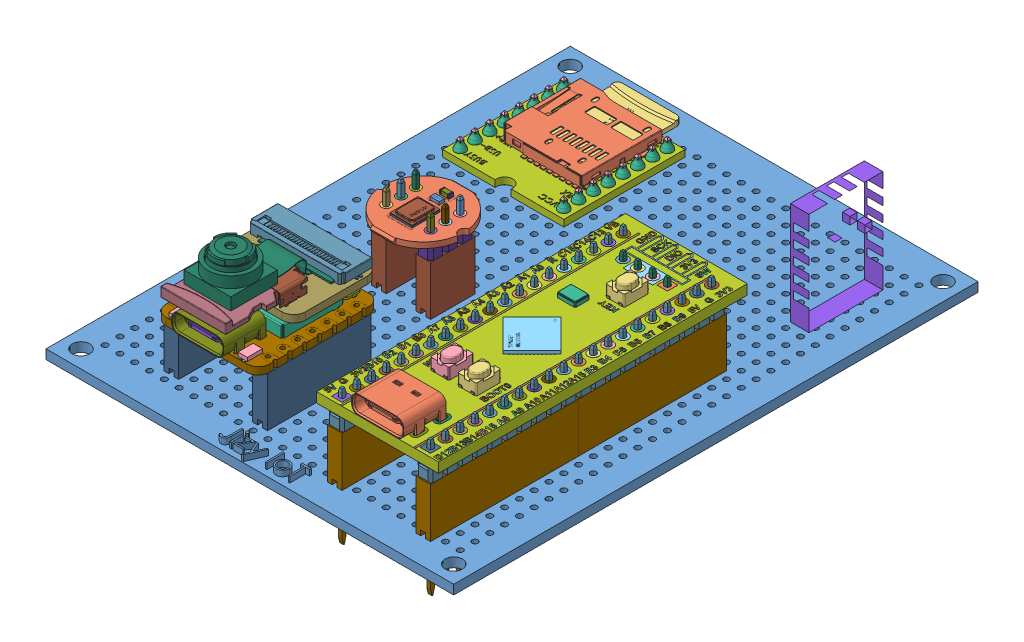
SolidWorks assembly 3D_Final, configuration Default. Lengths in mm.
Overall size (70 34.34 90).
331 component instances, 245 part files, 43 mates.
Components (placement in the parent):
- BoardDong7x9-1: BoardDong7x9 [Default] at (35 1.6 45) x (0 0 -1) z (0 1 0) size (90 70 2.6)
- blackpill v2.0 swi.STEP-1: blackpill v2.0 swi.STEP [Default] at (52.8 12.64 59.37) x (0 0 -1) z (0 1 0) size (53 20.9 10.45)
  - blackpill v2.0.step.STEP-1: blackpill v2.0.step.STEP [Default] at origin size (53 20.9 4.92)
    - USB Type C Port (SMD Type).step.STEP-1: USB Type C Port (SMD Type).step.STEP [Default] at (-19.2 0 3.305) x (0 -1 0) z (0 0 -1) size (8.94 7.9 4.2)
    - PTS810 SJK 250 SMTR LFS--3DModel-STEP-1.step.STEP-1: PTS810 SJK 250 SMTR LFS--3DModel-STEP-1.step.STEP [Default] at (14.5 -1.8498 1.7) x (1 0 0) z (0 -1 0) size (4.6 2.51 3.2)
    - PTS810 SJK 250 SMTR LFS--3DModel-STEP-1.step.STEP-2: PTS810 SJK 250 SMTR LFS--3DModel-STEP-1.step.STEP [Default] at (-11.4 -2.3498 1.7) x (1 0 0) z (0 -1 0) size (4.6 2.51 3.2)
    - PTS810 SJK 250 SMTR LFS--3DModel-STEP-1 v2(Mirror).step.STEP-1: PTS810 SJK 250 SMTR LFS--3DModel-STEP-1 v2(Mirror).step.STEP [Default] at (-11.4 2.3498 1.7) x (1 0 0) z (0 -1 0) size (4.6 2.51 3.2)
    - STM32F411CEU6.step.STEP-1: STM32F411CEU6.step.STEP [Default] at (0 0 1.7) x (-0.707107 -0.707107 0) z (-0.707107 0.707107 0) size (7 0.6 7)
    - ECS-135.60-12-33Q-JES-TR.step.STEP-1: ECS-135.60-12-33Q-JES-TR.step.STEP [Default] at (9.3867 2.3215 1.7) x (0 -1 0) z (-1 0 0) size (3.2 0.8 2.5)
    - DIY_black_pill.step.STEP-1: DIY_black_pill.step.STEP [Default] at origin size (53 20.9 1.7)
    - DIY_black_pill-0.step.STEP-1: DIY_black_pill-0.step.STEP [Default] at origin size (1.8 1.8 1.72)
    - DIY_black_pill-1.step.STEP-1: DIY_black_pill-1.step.STEP [Default] at origin size (1.8 1.8 1.72)
    - DIY_black_pill-2.step.STEP-1: DIY_black_pill-2.step.STEP [Default] at origin size (1.8 1.8 1.72)
    - DIY_black_pill-3.step.STEP-1: DIY_black_pill-3.step.STEP [Default] at origin size (1.8 1.8 1.72)
    - DIY_black_pill-4.step.STEP-1: DIY_black_pill-4.step.STEP [Default] at origin size (1.8 1.8 1.72)
    - DIY_black_pill-5.step.STEP-1: DIY_black_pill-5.step.STEP [Default] at origin size (1.8 1.8 1.72)
    - DIY_black_pill-6.step.STEP-1: DIY_black_pill-6.step.STEP [Default] at origin size (1.8 1.8 1.72)
    - DIY_black_pill-7.step.STEP-1: DIY_black_pill-7.step.STEP [Default] at origin size (1.8 1.8 1.72)
    - DIY_black_pill-8.step.STEP-1: DIY_black_pill-8.step.STEP [Default] at origin size (1.8 1.8 1.72)
    - DIY_black_pill-9.step.STEP-1: DIY_black_pill-9.step.STEP [Default] at origin size (1.8 1.8 1.72)
    - DIY_black_pill-10.step.STEP-1: DIY_black_pill-10.step.STEP [Default] at origin size (1.8 1.8 1.72)
    - DIY_black_pill-11.step.STEP-1: DIY_black_pill-11.step.STEP [Default] at origin size (1.8 1.8 1.72)
    - DIY_black_pill-12.step.STEP-1: DIY_black_pill-12.step.STEP [Default] at origin size (1.8 1.8 1.72)
    - DIY_black_pill-13.step.STEP-1: DIY_black_pill-13.step.STEP [Default] at origin size (1.8 1.8 1.72)
    - DIY_black_pill-14.step.STEP-1: DIY_black_pill-14.step.STEP [Default] at origin size (1.8 1.8 1.72)
    - DIY_black_pill-15.step.STEP-1: DIY_black_pill-15.step.STEP [Default] at origin size (1.8 1.8 1.72)
    - DIY_black_pill-16.step.STEP-1: DIY_black_pill-16.step.STEP [Default] at origin size (1.8 1.8 1.72)
    - DIY_black_pill-17.step.STEP-1: DIY_black_pill-17.step.STEP [Default] at origin size (1.8 1.8 1.72)
    - DIY_black_pill-18.step.STEP-1: DIY_black_pill-18.step.STEP [Default] at origin size (1.8 1.8 1.72)
    - DIY_black_pill-19.step.STEP-1: DIY_black_pill-19.step.STEP [Default] at origin size (1.8 1.8 1.72)
    - DIY_black_pill-20.step.STEP-1: DIY_black_pill-20.step.STEP [Default] at origin size (1.8 1.8 1.72)
    - DIY_black_pill-21.step.STEP-1: DIY_black_pill-21.step.STEP [Default] at origin size (1.8 1.8 1.72)
    - DIY_black_pill-22.step.STEP-1: DIY_black_pill-22.step.STEP [Default] at origin size (1.8 1.8 1.72)
    - DIY_black_pill-23.step.STEP-1: DIY_black_pill-23.step.STEP [Default] at origin size (1.8 1.8 1.72)
    - DIY_black_pill-24.step.STEP-1: DIY_black_pill-24.step.STEP [Default] at origin size (1.8 1.8 1.72)
    - DIY_black_pill-25.step.STEP-1: DIY_black_pill-25.step.STEP [Default] at origin size (1.8 1.8 1.72)
    - DIY_black_pill-26.step.STEP-1: DIY_black_pill-26.step.STEP [Default] at origin size (1.8 1.8 1.72)
    - DIY_black_pill-27.step.STEP-1: DIY_black_pill-27.step.STEP [Default] at origin size (1.8 1.8 1.72)
    - DIY_black_pill-28.step.STEP-1: DIY_black_pill-28.step.STEP [Default] at origin size (1.8 1.8 1.72)
    - DIY_black_pill-29.step.STEP-1: DIY_black_pill-29.step.STEP [Default] at origin size (1.8 1.8 1.72)
    - DIY_black_pill-30.step.STEP-1: DIY_black_pill-30.step.STEP [Default] at origin size (1.8 1.8 1.72)
    - DIY_black_pill-31.step.STEP-1: DIY_black_pill-31.step.STEP [Default] at origin size (1.8 1.8 1.72)
    - DIY_black_pill-32.step.STEP-1: DIY_black_pill-32.step.STEP [Default] at origin size (1.8 1.8 1.72)
    - DIY_black_pill-33.step.STEP-1: DIY_black_pill-33.step.STEP [Default] at origin size (1.8 1.8 1.72)
    - DIY_black_pill-34.step.STEP-1: DIY_black_pill-34.step.STEP [Default] at origin size (1.8 1.8 1.72)
    - DIY_black_pill-35.step.STEP-1: DIY_black_pill-35.step.STEP [Default] at origin size (1.8 1.8 1.72)
    - DIY_black_pill-36.step.STEP-1: DIY_black_pill-36.step.STEP [Default] at origin size (1.8 1.8 1.72)
    - DIY_black_pill-37.step.STEP-1: DIY_black_pill-37.step.STEP [Default] at origin size (1.8 1.8 1.72)
    - DIY_black_pill-38.step.STEP-1: DIY_black_pill-38.step.STEP [Default] at origin size (1.8 1.8 1.72)
    - DIY_black_pill-39.step.STEP-1: DIY_black_pill-39.step.STEP [Default] at origin size (1.8 1.8 1.72)
    - DIY_black_pill-40.step.STEP-1: DIY_black_pill-40.step.STEP [Default] at origin size (51.2 0.3 0.01)
    - DIY_black_pill-41.step.STEP-1: DIY_black_pill-41.step.STEP [Default] at origin size (51.2 0.3 0.01)
    - DIY_black_pill-42.step.STEP-1: DIY_black_pill-42.step.STEP [Default] at origin size (0.93 1 0.01)
    - DIY_black_pill-43.step.STEP-1: DIY_black_pill-43.step.STEP [Default] at origin size (0.94 1.03 0.01)
    - DIY_black_pill-44.step.STEP-1: DIY_black_pill-44.step.STEP [Default] at origin size (0.93 1 0.01)
    - DIY_black_pill-45.step.STEP-1: DIY_black_pill-45.step.STEP [Default] at origin size (0.67 1.02 0.01)
    - DIY_black_pill-46.step.STEP-1: DIY_black_pill-46.step.STEP [Default] at origin size (0.66 1.02 0.01)
    - DIY_black_pill-47.step.STEP-1: DIY_black_pill-47.step.STEP [Default] at origin size (0.84 1 0.01)
    - DIY_black_pill-48.step.STEP-1: DIY_black_pill-48.step.STEP [Default] at origin size (0.67 1.02 0.01)
    - DIY_black_pill-49.step.STEP-1: DIY_black_pill-49.step.STEP [Default] at origin size (0.84 1.01 0.01)
    - DIY_black_pill-50.step.STEP-1: DIY_black_pill-50.step.STEP [Default] at origin size (0.72 1.01 0.01)
    - DIY_black_pill-51.step.STEP-1: DIY_black_pill-51.step.STEP [Default] at origin size (0.84 1 0.01)
    - DIY_black_pill-52.step.STEP-1: DIY_black_pill-52.step.STEP [Default] at origin size (0.67 1 0.01)
    - DIY_black_pill-53.step.STEP-1: DIY_black_pill-53.step.STEP [Default] at origin size (1 1 0.01)
    - DIY_black_pill-54.step.STEP-1: DIY_black_pill-54.step.STEP [Default] at origin size (0.44 1 0.01)
    - DIY_black_pill-55.step.STEP-1: DIY_black_pill-55.step.STEP [Default] at origin size (0.44 1 0.01)
    - DIY_black_pill-56.step.STEP-1: DIY_black_pill-56.step.STEP [Default] at origin size (1 1 0.01)
    - DIY_black_pill-57.step.STEP-1: DIY_black_pill-57.step.STEP [Default] at origin size (0.44 1 0.01)
    - DIY_black_pill-58.step.STEP-1: DIY_black_pill-58.step.STEP [Default] at origin size (0.67 1.02 0.01)
    - DIY_black_pill-59.step.STEP-1: DIY_black_pill-59.step.STEP [Default] at origin size (0.66 1.02 0.01)
    - DIY_black_pill-60.step.STEP-1: DIY_black_pill-60.step.STEP [Default] at origin size (0.67 1 0.01)
    - DIY_black_pill-61.step.STEP-1: DIY_black_pill-61.step.STEP [Default] at origin size (0.84 1 0.01)
    - DIY_black_pill-62.step.STEP-1: DIY_black_pill-62.step.STEP [Default] at origin size (0.44 1 0.01)
    - DIY_black_pill-63.step.STEP-1: DIY_black_pill-63.step.STEP [Default] at origin size (0.66 1.02 0.01)
    - DIY_black_pill-64.step.STEP-1: DIY_black_pill-64.step.STEP [Default] at origin size (0.44 1 0.01)
    - DIY_black_pill-65.step.STEP-1: DIY_black_pill-65.step.STEP [Default] at origin size (0.84 1 0.01)
    - DIY_black_pill-66.step.STEP-1: DIY_black_pill-66.step.STEP [Default] at origin size (0.72 1 0.01)
    - DIY_black_pill-67.step.STEP-1: DIY_black_pill-67.step.STEP [Default] at origin size (0.44 1 0.01)
    - DIY_black_pill-68.step.STEP-1: DIY_black_pill-68.step.STEP [Default] at origin size (0.84 1 0.01)
    - DIY_black_pill-69.step.STEP-1: DIY_black_pill-69.step.STEP [Default] at origin size (1 1 0.01)
    - DIY_black_pill-70.step.STEP-1: DIY_black_pill-70.step.STEP [Default] at origin size (1 1 0.01)
    - DIY_black_pill-71.step.STEP-1: DIY_black_pill-71.step.STEP [Default] at origin size (0.65 1.02 0.01)
    - DIY_black_pill-72.step.STEP-1: DIY_black_pill-72.step.STEP [Default] at origin size (0.44 1 0.01)
    - DIY_black_pill-73.step.STEP-1: DIY_black_pill-73.step.STEP [Default] at origin size (1 1 0.01)
    - DIY_black_pill-74.step.STEP-1: DIY_black_pill-74.step.STEP [Default] at origin size (0.67 1 0.01)
    - DIY_black_pill-75.step.STEP-1: DIY_black_pill-75.step.STEP [Default] at origin size (0.44 1 0.01)
    - DIY_black_pill-76.step.STEP-1: DIY_black_pill-76.step.STEP [Default] at origin size (1 1 0.01)
    - DIY_black_pill-77.step.STEP-1: DIY_black_pill-77.step.STEP [Default] at origin size (0.66 1.02 0.01)
    - DIY_black_pill-78.step.STEP-1: DIY_black_pill-78.step.STEP [Default] at origin size (0.84 1.01 0.01)
    - DIY_black_pill-79.step.STEP-1: DIY_black_pill-79.step.STEP [Default] at origin size (0.67 1.01 0.01)
    - DIY_black_pill-80.step.STEP-1: DIY_black_pill-80.step.STEP [Default] at origin size (0.84 1 0.01)
    - DIY_black_pill-81.step.STEP-1: DIY_black_pill-81.step.STEP [Default] at origin size (0.66 0.99 0.01)
    - DIY_black_pill-82.step.STEP-1: DIY_black_pill-82.step.STEP [Default] at origin size (0.84 1 0.01)
    - DIY_black_pill-83.step.STEP-1: DIY_black_pill-83.step.STEP [Default] at origin size (0.84 1 0.01)
    - DIY_black_pill-84.step.STEP-1: DIY_black_pill-84.step.STEP [Default] at origin size (0.67 1 0.01)
    - DIY_black_pill-85.step.STEP-1: DIY_black_pill-85.step.STEP [Default] at origin size (0.66 1.02 0.01)
    - DIY_black_pill-86.step.STEP-1: DIY_black_pill-86.step.STEP [Default] at origin size (0.66 1.02 0.01)
    - DIY_black_pill-87.step.STEP-1: DIY_black_pill-87.step.STEP [Default] at origin size (0.67 1 0.01)
    - DIY_black_pill-88.step.STEP-1: DIY_black_pill-88.step.STEP [Default] at origin size (0.44 1 0.01)
    - DIY_black_pill-89.step.STEP-1: DIY_black_pill-89.step.STEP [Default] at origin size (0.84 1 0.01)
    - DIY_black_pill-90.step.STEP-1: DIY_black_pill-90.step.STEP [Default] at origin size (1 1 0.01)
    - DIY_black_pill-91.step.STEP-1: DIY_black_pill-91.step.STEP [Default] at origin size (0.84 1 0.01)
    - DIY_black_pill-92.step.STEP-1: DIY_black_pill-92.step.STEP [Default] at origin size (0.44 1 0.01)
    - DIY_black_pill-93.step.STEP-1: DIY_black_pill-93.step.STEP [Default] at origin size (0.87 1.03 0.01)
    - DIY_black_pill-94.step.STEP-1: DIY_black_pill-94.step.STEP [Default] at origin size (0.44 1 0.01)
    - DIY_black_pill-95.step.STEP-1: DIY_black_pill-95.step.STEP [Default] at origin size (0.44 1 0.01)
    - DIY_black_pill-96.step.STEP-1: DIY_black_pill-96.step.STEP [Default] at origin size (0.9 1 0.01)
    - DIY_black_pill-97.step.STEP-1: DIY_black_pill-97.step.STEP [Default] at origin size (0.65 1.02 0.01)
    - DIY_black_pill-98.step.STEP-1: DIY_black_pill-98.step.STEP [Default] at origin size (1 1 0.01)
    - DIY_black_pill-99.step.STEP-1: DIY_black_pill-99.step.STEP [Default] at origin size (0.72 1 0.01)
    - DIY_black_pill-100.step.STEP-1: DIY_black_pill-100.step.STEP [Default] at origin size (1 1 0.01)
    - DIY_black_pill-101.step.STEP-1: DIY_black_pill-101.step.STEP [Default] at origin size (0.67 1.02 0.01)
    - DIY_black_pill-102.step.STEP-1: DIY_black_pill-102.step.STEP [Default] at origin size (0.65 1.02 0.01)
    - DIY_black_pill-103.step.STEP-1: DIY_black_pill-103.step.STEP [Default] at origin size (1 1 0.01)
    - DIY_black_pill-104.step.STEP-1: DIY_black_pill-104.step.STEP [Default] at origin size (0.84 1 0.01)
    - DIY_black_pill-105.step.STEP-1: DIY_black_pill-105.step.STEP [Default] at origin size (0.84 1 0.01)
    - DIY_black_pill-106.step.STEP-1: DIY_black_pill-106.step.STEP [Default] at origin size (0.65 1.02 0.01)
    - DIY_black_pill-107.step.STEP-1: DIY_black_pill-107.step.STEP [Default] at origin size (0.66 1.02 0.01)
    - DIY_black_pill-108.step.STEP-1: DIY_black_pill-108.step.STEP [Default] at origin size (0.66 1.02 0.01)
    - DIY_black_pill-109.step.STEP-1: DIY_black_pill-109.step.STEP [Default] at origin size (0.67 1 0.01)
    - DIY_black_pill-110.step.STEP-1: DIY_black_pill-110.step.STEP [Default] at origin size (0.93 1 0.01)
    - DIY_black_pill-111.step.STEP-1: DIY_black_pill-111.step.STEP [Default] at origin size (0.94 1.03 0.01)
    - DIY_black_pill-112.step.STEP-1: DIY_black_pill-112.step.STEP [Default] at origin size (0.93 1 0.01)
    - DIY_black_pill-113.step.STEP-1: DIY_black_pill-113.step.STEP [Default] at origin size (0.44 1 0.01)
    - DIY_black_pill-114.step.STEP-1: DIY_black_pill-114.step.STEP [Default] at origin size (0.84 1 0.01)
    - DIY_black_pill-115.step.STEP-1: DIY_black_pill-115.step.STEP [Default] at origin size (0.67 1 0.01)
    - DIY_black_pill-116.step.STEP-1: DIY_black_pill-116.step.STEP [Default] at origin size (0.44 1 0.01)
    - DIY_black_pill-117.step.STEP-1: DIY_black_pill-117.step.STEP [Default] at origin size (0.66 0.99 0.01)
    - DIY_black_pill-118.step.STEP-1: DIY_black_pill-118.step.STEP [Default] at origin size (0.84 1 0.01)
    - DIY_black_pill-119.step.STEP-1: DIY_black_pill-119.step.STEP [Default] at origin size (1 1 0.01)
    - DIY_black_pill-120.step.STEP-1: DIY_black_pill-120.step.STEP [Default] at origin size (0.67 1 0.01)
    - DIY_black_pill-121.step.STEP-1: DIY_black_pill-121.step.STEP [Default] at origin size (1 1 0.01)
    - DIY_black_pill-122.step.STEP-1: DIY_black_pill-122.step.STEP [Default] at origin size (0.66 1.02 0.01)
    - DIY_black_pill-123.step.STEP-1: DIY_black_pill-123.step.STEP [Default] at origin size (1 1 0.01)
    - DIY_black_pill-124.step.STEP-1: DIY_black_pill-124.step.STEP [Default] at origin size (0.67 1 0.01)
    - DIY_black_pill-125.step.STEP-1: DIY_black_pill-125.step.STEP [Default] at origin size (0.87 1.03 0.01)
    - DIY_black_pill-126.step.STEP-1: DIY_black_pill-126.step.STEP [Default] at origin size (0.72 1 0.01)
    - DIY_black_pill-127.step.STEP-1: DIY_black_pill-127.step.STEP [Default] at origin size (0.66 1.02 0.01)
    - DIY_black_pill-128.step.STEP-1: DIY_black_pill-128.step.STEP [Default] at origin size (0.87 1.03 0.01)
    - DIY_black_pill-129.step.STEP-1: DIY_black_pill-129.step.STEP [Default] at origin size (0.93 1 0.01)
    - DIY_black_pill-130.step.STEP-1: DIY_black_pill-130.step.STEP [Default] at origin size (0.44 1 0.01)
    - DIY_black_pill-131.step.STEP-1: DIY_black_pill-131.step.STEP [Default] at origin size (2.55 1.5 1.72)
    - DIY_black_pill-132.step.STEP-1: DIY_black_pill-132.step.STEP [Default] at origin size (2.6 1.5 1.72)
    - DIY_black_pill-133.step.STEP-1: DIY_black_pill-133.step.STEP [Default] at origin size (2.55 1.5 1.72)
    - DIY_black_pill-134.step.STEP-1: DIY_black_pill-134.step.STEP [Default] at origin size (2.6 1.5 1.72)
    - DIY_black_pill-135.step.STEP-1: DIY_black_pill-135.step.STEP [Default] at origin size (1 1 0.01)
    - DIY_black_pill-136.step.STEP-1: DIY_black_pill-136.step.STEP [Default] at origin size (0.67 1.01 0.01)
    - DIY_black_pill-137.step.STEP-1: DIY_black_pill-137.step.STEP [Default] at origin size (1.8 1.8 1.72)
    - DIY_black_pill-138.step.STEP-1: DIY_black_pill-138.step.STEP [Default] at origin size (1.8 1.8 1.72)
    - DIY_black_pill-139.step.STEP-1: DIY_black_pill-139.step.STEP [Default] at origin size (1.8 1.8 1.72)
    - DIY_black_pill-140.step.STEP-1: DIY_black_pill-140.step.STEP [Default] at origin size (1.8 1.8 1.72)
    - DIY_black_pill-141.step.STEP-1: DIY_black_pill-141.step.STEP [Default] at origin size (8.17 10.16 0.01)
    - DIY_black_pill-142.step.STEP-1: DIY_black_pill-142.step.STEP [Default] at origin size (1.31 1 0.01)
    - DIY_black_pill-143.step.STEP-1: DIY_black_pill-143.step.STEP [Default] at origin size (0.93 1 0.01)
    - DIY_black_pill-144.step.STEP-1: DIY_black_pill-144.step.STEP [Default] at origin size (0.84 1 0.01)
    - DIY_black_pill-145.step.STEP-1: DIY_black_pill-145.step.STEP [Default] at origin size (0.2 1 0.01)
    - DIY_black_pill-146.step.STEP-1: DIY_black_pill-146.step.STEP [Default] at origin size (0.87 1.03 0.01)
    - DIY_black_pill-147.step.STEP-1: DIY_black_pill-147.step.STEP [Default] at origin size (0.94 1.03 0.01)
    - DIY_black_pill-148.step.STEP-1: DIY_black_pill-148.step.STEP [Default] at origin size (0.79 1 0.01)
    - DIY_black_pill-149.step.STEP-1: DIY_black_pill-149.step.STEP [Default] at origin size (0.84 1 0.01)
    - DIY_black_pill-150.step.STEP-1: DIY_black_pill-150.step.STEP [Default] at origin size (0.9 1 0.01)
    - DIY_black_pill-151.step.STEP-1: DIY_black_pill-151.step.STEP [Default] at origin size (0.81 1.03 0.01)
    - DIY_black_pill-152.step.STEP-1: DIY_black_pill-152.step.STEP [Default] at origin size (0.97 1.03 0.01)
    - DIY_black_pill-153.step.STEP-1: DIY_black_pill-153.step.STEP [Default] at origin size (0.66 1.02 0.01)
    - DIY_black_pill-154.step.STEP-1: DIY_black_pill-154.step.STEP [Default] at origin size (0.66 1.02 0.01)
    - DIY_black_pill-155.step.STEP-1: DIY_black_pill-155.step.STEP [Default] at origin size (0.81 1.03 0.01)
    - DIY_black_pill-156.step.STEP-1: DIY_black_pill-156.step.STEP [Default] at origin size (0.9 1 0.01)
    - DIY_black_pill-157.step.STEP-1: DIY_black_pill-157.step.STEP [Default] at origin size (0.81 1.03 0.01)
    - DIY_black_pill-158.step.STEP-1: DIY_black_pill-158.step.STEP [Default] at origin size (0.97 1.03 0.01)
    - DIY_black_pill-159.step.STEP-1: DIY_black_pill-159.step.STEP [Default] at origin size (0.97 1.03 0.01)
    - DIY_black_pill-160.step.STEP-1: DIY_black_pill-160.step.STEP [Default] at origin size (1.01 0.91 0.01)
    - DIY_black_pill-161.step.STEP-1: DIY_black_pill-161.step.STEP [Default] at origin size (1 0.94 0.01)
    - DIY_black_pill-162.step.STEP-1: DIY_black_pill-162.step.STEP [Default] at origin size (1 0.77 0.01)
    - DIY_black_pill-163.step.STEP-1: DIY_black_pill-163.step.STEP [Default] at origin size (0.79 1 0.01)
    - DIY_black_pill-164.step.STEP-1: DIY_black_pill-164.step.STEP [Default] at origin size (0.65 1.02 0.01)
    - DIY_black_pill-165.step.STEP-1: DIY_black_pill-165.step.STEP [Default] at origin size (0.84 1 0.01)
    - DIY_black_pill-166.step.STEP-1: DIY_black_pill-166.step.STEP [Default] at origin size (0.79 1 0.01)
    - DIY_black_pill-167.step.STEP-1: DIY_black_pill-167.step.STEP [Default] at origin size (0.79 1 0.01)
  - 1x20 Male Pin Header.STEP-1: 1x20 Male Pin Header.STEP [Default] at (23.26 -7.6 0) x (-1 0 0) z (0 -1 0) size (50.8 8.54 2.5)
  - 1x20 Male Pin Header.STEP-2: 1x20 Male Pin Header.STEP [Default] at (23.26 7.6 0) x (-1 0 0) z (0 -1 0) size (50.8 8.54 2.5)
  - 1x4 Male Pin Header.STEP-1: 1x4 Male Pin Header.STEP [Default] at (19.45 -3.81 0) x (0 1 0) z (-1 0 0) size (10.17 8.54 2.5)
- Seeed Studio XIAO-ESP32-S3-Sense-1: Seeed Studio XIAO-ESP32-S3-Sense [Default] at (16.1886 10.35 72.4693) x (0 0 1) z (-1 0 0) size (24.36 13.98 17.79)
  - Seeed Studio XIAO-ESP32-S3-Sense.step-1: Seeed Studio XIAO-ESP32-S3-Sense.step [Default] at origin size (24.36 13.98 17.79)
    - Seeed Studio XIAO-ESP32-S3 (Sense).step-1: Seeed Studio XIAO-ESP32-S3 (Sense).step [Default] at origin size (22.49 4.48 17.79)
      - USB TYPE C PORT.step-1: USB TYPE C PORT.step [Default] at (4.3161 13.395 -12.1571) x (0 0 -1) z (0 -1 0) size (8.94 7.9 4.2)
        - USB TYPE C PORT (1).step-1: USB TYPE C PORT (1).step [Default] at (-3.0192 1.0963 5.395) size (8.94 7.9 4.2)
          - BOSS-EXTRUDE14_8_.step-1: BOSS-EXTRUDE14_8_.step [Default] at (-3.0192 1.0963 5.395) size (0.6 1 0.3)
          - BOSS-EXTRUDE7_4_.step-1: BOSS-EXTRUDE7_4_.step [Default] at (-3.0192 1.0963 5.395) size (0.3 3.78 0.75)
          - BOSS-EXTRUDE7_3_.step-1: BOSS-EXTRUDE7_3_.step [Default] at (-3.0192 1.0963 5.395) size (0.3 3.78 0.75)
          - BOSS-EXTRUDE14_4_.step-1: BOSS-EXTRUDE14_4_.step [Default] at (-3.0192 1.0963 5.395) size (0.3 1 0.3)
          - BOSS-EXTRUDE14_2_.step-1: BOSS-EXTRUDE14_2_.step [Default] at (-3.0192 1.0963 5.395) size (0.6 1 0.3)
          - BOSS-EXTRUDE14_11_.step-1: BOSS-EXTRUDE14_11_.step [Default] at (-3.0192 1.0963 5.395) size (0.3 1 0.3)
          - BOSS-EXTRUDE7_7_.step-1: BOSS-EXTRUDE7_7_.step [Default] at (-3.0192 1.0963 5.395) size (0.3 3.78 0.75)
          - BOSS-EXTRUDE14_9_.step-1: BOSS-EXTRUDE14_9_.step [Default] at (-3.0192 1.0963 5.395) size (0.3 1 0.3)
          - BOSS-EXTRUDE14_3_.step-1: BOSS-EXTRUDE14_3_.step [Default] at (-3.0192 1.0963 5.395) size (0.3 1 0.3)
          - BOSS-EXTRUDE14_7_.step-1: BOSS-EXTRUDE14_7_.step [Default] at (-3.0192 1.0963 5.395) size (0.6 1 0.3)
          - MIRROR2.step-1: MIRROR2.step [Default] at (-3.0192 1.0963 5.395) size (6.7 4.6 0.7)
          - BOSS-EXTRUDE14_5_.step-1: BOSS-EXTRUDE14_5_.step [Default] at (-3.0192 1.0963 5.395) size (0.3 1 0.3)
          - BOSS-EXTRUDE14_12_.step-1: BOSS-EXTRUDE14_12_.step [Default] at (-3.0192 1.0963 5.395) size (0.3 1 0.3)
          - BOSS-EXTRUDE7_8_.step-1: BOSS-EXTRUDE7_8_.step [Default] at (-3.0192 1.0963 5.395) size (0.3 3.78 0.75)
          - BOSS-EXTRUDE7_1_.step-1: BOSS-EXTRUDE7_1_.step [Default] at (-3.0192 1.0963 5.395) size (0.3 3.78 0.75)
          - BOSS-EXTRUDE14_10_.step-1: BOSS-EXTRUDE14_10_.step [Default] at (-3.0192 1.0963 5.395) size (0.3 1 0.3)
          - BOSS-EXTRUDE7_9_.step-1: BOSS-EXTRUDE7_9_.step [Default] at (-3.0192 1.0963 5.395) size (0.3 3.78 0.75)
          - BOSS-EXTRUDE14_6_.step-1: BOSS-EXTRUDE14_6_.step [Default] at (-3.0192 1.0963 5.395) size (0.6 1 0.3)
          - CHAMFER9.step-1: CHAMFER9.step [Default] at (-3.0192 1.0963 5.395) size (8.94 7.3 4.2)
          - BOSS-EXTRUDE14_1_.step-1: BOSS-EXTRUDE14_1_.step [Default] at (-3.0192 1.0963 5.395) size (0.3 1 0.3)
          - BOSS-EXTRUDE7_6_.step-1: BOSS-EXTRUDE7_6_.step [Default] at (-3.0192 1.0963 5.395) size (0.3 3.78 0.75)
          - BOSS-EXTRUDE7_2_.step-1: BOSS-EXTRUDE7_2_.step [Default] at (-3.0192 1.0963 5.395) size (0.3 3.78 0.75)
          - CUT-EXTRUDE5.step-1: CUT-EXTRUDE5.step [Default] at (-3.0192 1.0963 5.395) size (8.54 2 3.59)
          - BOSS-EXTRUDE7_5_.step-1: BOSS-EXTRUDE7_5_.step [Default] at (-3.0192 1.0963 5.395) size (0.3 3.78 0.75)
      - SKTAAAE010 v1.step-1: SKTAAAE010 v1.step [Default] at (10.7092 1 -12.0449) x (1 0 0) z (0 1 0) size (3.09 1.6 0.73)
        - Body.step-1: Body.step [Default] at (0 0 0.1) size (2.6 1.6 0.63)
        - Pins.step-1: Pins.step [Default] at origin size (3.09 1.19 0.1)
      - SKTAAAE010 v1.step-2: SKTAAAE010 v1.step [Default] at (10.6911 1 -0.1868) x (1 0 0) z (0 1 0) size (3.09 1.6 0.73)
        - Body.step-1: Body.step [Default] at (0 0 0.1) size (2.6 1.6 0.63)
        - Pins.step-1: Pins.step [Default] at origin size (3.09 1.19 0.1)
      - Shield.step-1: Shield.step [Default] at origin size (10.6 2.7 12.6)
      - U.FL-R-SMT-1_10_ v1.step-1: U.FL-R-SMT-1_10_ v1.step [Default] at (-6.9517 1 -10.8381) x (1 0 0) z (0 1 0) size (3 3.1 1.25)
      - DF40C-30DP-0.4V_51_ v1.step-1: DF40C-30DP-0.4V_51_ v1.step [Default] at (-6.0667 1.65 -7.7227) size (2.97 1.14 7.52)
      - Seeed Studio XIAO-ESP32-S3 (Sense)-0.step-1: Seeed Studio XIAO-ESP32-S3 (Sense)-0.step [Default] at origin size (20.97 1.28 17.79)
    - Sense Expansion Board.step-1: Sense Expansion Board.step [Default] at (-0.3 4.5 0) x (-1 0 0) z (0 0 1) size (24.36 7.23 16.78)
      - DF40HC(3.0)-30DS.step-1: DF40HC(3.0)-30DS.step [Default] at (6.4217 1.57 -3.0777) x (-1 0 0) z (0 0 1) size (3.38 2.9 8.6)
      - 10067099-200LF v1.step-1: 10067099-200LF v1.step [Default] at (-1.3077 -2.08 -6.0846) x (0 0 -1) z (-1 0 0) size (11.4 2.65 5.5)
      - PCB.step-1: PCB.step [Default] at origin size (14.68 1.25 16.78)
      - MicroSD v2.step-1: MicroSD v2.step [Default] at (-8.16 -2.1 -6.9267) x (1 0 0) z (0 0 -1) size (15.06 1.66 11.19)
      - JUSHUO AFC01-S24FCA-00.step-1: JUSHUO AFC01-S24FCA-00.step [Default] at (6.9932 -0.67 -6.0797) x (0 0 1) z (0 -1 0) size (16.2 6.01 2.01)
    - Camer Module.step-1: Camer Module.step [Default] at (-7.2 6 -13) size (19.95 8.11 12.5)
- INMP441 I2S Microphone Module v15-1: INMP441 I2S Microphone Module v15 [Default] at (23.57 12.61 48.81) size (13.77 11.25 14.24)
  - INMP441 I2S Microphone Module v15.step-1: INMP441 I2S Microphone Module v15.step [Default] at origin size (13.77 11.25 14.24)
    - C0603_070.step-1: C0603_070.step [Default] at (0 8.5 0) x (1 0 0) z (0 1 0) size (1.6 0.8 0.7)
      - C0603_070_1.step-1: C0603_070_1.step [Default] at origin size (1.6 0.8 0.7)
        - Part 3.step-1: Part 3.step [Default] at (0 4 -7.535) size (1.4 0.77 0.67)
        - Part 2.step-1: Part 2.step [Default] at (0 4 -7.535) size (0.2 0.8 0.7)
        - Part 1.step-1: Part 1.step [Default] at (0 4 -7.535) size (0.2 0.8 0.7)
    - 0603 Resistor.step-1: 0603 Resistor.step [Default] at (0 0.98 -2.4) x (1 0 0) z (0 1 0) size (1.6 0.9 0.5)
    - INMP441 I2S Microphone Module.step-1: INMP441 I2S Microphone Module.step [Default] at origin size (13.77 1 14.24)
    - INMP441 I2S Microphone Module-0.step-1: INMP441 I2S Microphone Module-0.step [Default] at origin size (1.6 1 1.6)
    - INMP441 I2S Microphone Module-1.step-1: INMP441 I2S Microphone Module-1.step [Default] at origin size (1.6 1 1.6)
    - INMP441 I2S Microphone Module-2.step-1: INMP441 I2S Microphone Module-2.step [Default] at origin size (1.6 1 1.6)
    - INMP441 I2S Microphone Module-3.step-1: INMP441 I2S Microphone Module-3.step [Default] at origin size (1.6 1 1.6)
    - INMP441 I2S Microphone Module-4.step-1: INMP441 I2S Microphone Module-4.step [Default] at origin size (1.6 1 1.6)
    - INMP441 I2S Microphone Module-5.step-1: INMP441 I2S Microphone Module-5.step [Default] at origin size (1.6 1 1.6)
    - INMP441 I2S Microphone Module-6.step-1: INMP441 I2S Microphone Module-6.step [Default] at origin size (1.6 1 1.6)
    - INMP441 I2S Microphone Module-7.step-1: INMP441 I2S Microphone Module-7.step [Default] at origin size (3.79 0.3 4.79)
    - INMP441 I2S Microphone Module-8.step-1: INMP441 I2S Microphone Module-8.step [Default] at origin size (3.79 0.41 4.79)
    - INMP441 I2S Microphone Module-9.step-1: INMP441 I2S Microphone Module-9.step [Default] at origin size (0.65 11.25 0.65)
    - INMP441 I2S Microphone Module-10.step-1: INMP441 I2S Microphone Module-10.step [Default] at origin size (2.55 2.5 7.63)
    - INMP441 I2S Microphone Module-11.step-1: INMP441 I2S Microphone Module-11.step [Default] at origin size (0.65 11.25 0.65)
    - INMP441 I2S Microphone Module-12.step-1: INMP441 I2S Microphone Module-12.step [Default] at origin size (0.65 11.25 0.65)
    - INMP441 I2S Microphone Module-13.step-1: INMP441 I2S Microphone Module-13.step [Default] at origin size (0.65 11.25 0.65)
    - INMP441 I2S Microphone Module-14.step-1: INMP441 I2S Microphone Module-14.step [Default] at origin size (2.55 2.5 7.63)
    - INMP441 I2S Microphone Module-15.step-1: INMP441 I2S Microphone Module-15.step [Default] at origin size (0.65 11.25 0.65)
    - INMP441 I2S Microphone Module-16.step-1: INMP441 I2S Microphone Module-16.step [Default] at origin size (0.65 11.25 0.65)
- DFPlayer Mini Assem v1.step-1: DFPlayer Mini Assem v1.step [Default] at (15.95 1.6 17.06) x (-1 0 0) z (0 0 -1) size (20.8 11.2 23.46)
  - SD card Assem^DFPlayer Mini Assem v1.step-1: SD card Assem^DFPlayer Mini Assem v1.step [Default] at (-198.0203 122.5536 -43.8714) x (0 1 0) z (1 0 0) size (2.44 17.9 16) (virtual)
    - CD card slot^SD card Assem_DFPlayer Mini Assem v1.step-1: CD card slot^SD card Assem_DFPlayer Mini Assem v1.step [Default] at (-120.5536 47.0914 197.6703) x (0 0 1) z (1 0 0) size (16 15 2.44) (virtual)
    - Micro sd card^SD card Assem_DFPlayer Mini Assem v1.step-1: Micro sd card^SD card Assem_DFPlayer Mini Assem v1.step [Default] at (-120.5536 45.5089 151.9853) x (0 0 1) z (1 0 0) size (11 15 0.95) (virtual)
  - DFPlayer Mini Pin.step-1: DFPlayer Mini Pin.step [Default] at (8.89 0 8.89) x (0 0 -1) z (0 -1 0) size (2.54 2.54 11.2)
    - 11_20mm pin.step-1: 11_20mm pin.step [Default] at (0 0 2.6) size (0.63 0.63 11.2)
    - Pin Header 1x12 TH Pitch 2.step-1: Pin Header 1x12 TH Pitch 2.step [Default] at (-27.94 0 -0.0014) size (2.54 2.54 2.8)
    - solder.step-1: solder.step [Default] at (0 0 -1.15) x (1 0 0) z (0 1 0) size (1.8 1.45 1.8)
  - DFPlayer Mini Pin.step-2: DFPlayer Mini Pin.step [Default] at (-8.89 0 8.89) x (0 0 1) z (0 -1 0) size (2.54 2.54 11.2)
    - 11_20mm pin.step-1: 11_20mm pin.step [Default] at (0 0 2.6) size (0.63 0.63 11.2)
    - Pin Header 1x12 TH Pitch 2.step-1: Pin Header 1x12 TH Pitch 2.step [Default] at (-27.94 0 -0.0014) size (2.54 2.54 2.8)
    - solder.step-1: solder.step [Default] at (0 0 -1.15) x (1 0 0) z (0 1 0) size (1.8 1.45 1.8)
  - DFPlayer Mini Pin.step-3: DFPlayer Mini Pin.step [Default] at (-8.89 0 6.35) x (0 0 1) z (0 -1 0) size (2.54 2.54 11.2)
    - 11_20mm pin.step-1: 11_20mm pin.step [Default] at (0 0 2.6) size (0.63 0.63 11.2)
    - Pin Header 1x12 TH Pitch 2.step-1: Pin Header 1x12 TH Pitch 2.step [Default] at (-27.94 0 -0.0014) size (2.54 2.54 2.8)
    - solder.step-1: solder.step [Default] at (0 0 -1.15) x (1 0 0) z (0 1 0) size (1.8 1.45 1.8)
  - DFPlayer Mini Pin.step-4: DFPlayer Mini Pin.step [Default] at (-8.89 0 3.81) x (0 0 1) z (0 -1 0) size (2.54 2.54 11.2)
    - 11_20mm pin.step-1: 11_20mm pin.step [Default] at (0 0 2.6) size (0.63 0.63 11.2)
    - Pin Header 1x12 TH Pitch 2.step-1: Pin Header 1x12 TH Pitch 2.step [Default] at (-27.94 0 -0.0014) size (2.54 2.54 2.8)
    - solder.step-1: solder.step [Default] at (0 0 -1.15) x (1 0 0) z (0 1 0) size (1.8 1.45 1.8)
  - DFPlayer Mini Pin.step-5: DFPlayer Mini Pin.step [Default] at (-8.89 0 1.27) x (0 0 1) z (0 -1 0) size (2.54 2.54 11.2)
    - 11_20mm pin.step-1: 11_20mm pin.step [Default] at (0 0 2.6) size (0.63 0.63 11.2)
    - Pin Header 1x12 TH Pitch 2.step-1: Pin Header 1x12 TH Pitch 2.step [Default] at (-27.94 0 -0.0014) size (2.54 2.54 2.8)
    - solder.step-1: solder.step [Default] at (0 0 -1.15) x (1 0 0) z (0 1 0) size (1.8 1.45 1.8)
  - DFPlayer Mini Pin.step-6: DFPlayer Mini Pin.step [Default] at (-8.89 0 -1.27) x (0 0 1) z (0 -1 0) size (2.54 2.54 11.2)
    - 11_20mm pin.step-1: 11_20mm pin.step [Default] at (0 0 2.6) size (0.63 0.63 11.2)
    - Pin Header 1x12 TH Pitch 2.step-1: Pin Header 1x12 TH Pitch 2.step [Default] at (-27.94 0 -0.0014) size (2.54 2.54 2.8)
    - solder.step-1: solder.step [Default] at (0 0 -1.15) x (1 0 0) z (0 1 0) size (1.8 1.45 1.8)
  - DFPlayer Mini Pin.step-7: DFPlayer Mini Pin.step [Default] at (-8.89 0 -3.81) x (0 0 1) z (0 -1 0) size (2.54 2.54 11.2)
    - 11_20mm pin.step-1: 11_20mm pin.step [Default] at (0 0 2.6) size (0.63 0.63 11.2)
    - Pin Header 1x12 TH Pitch 2.step-1: Pin Header 1x12 TH Pitch 2.step [Default] at (-27.94 0 -0.0014) size (2.54 2.54 2.8)
    - solder.step-1: solder.step [Default] at (0 0 -1.15) x (1 0 0) z (0 1 0) size (1.8 1.45 1.8)
  - DFPlayer Mini Pin.step-8: DFPlayer Mini Pin.step [Default] at (-8.89 0 -6.35) x (0 0 1) z (0 -1 0) size (2.54 2.54 11.2)
    - 11_20mm pin.step-1: 11_20mm pin.step [Default] at (0 0 2.6) size (0.63 0.63 11.2)
    - Pin Header 1x12 TH Pitch 2.step-1: Pin Header 1x12 TH Pitch 2.step [Default] at (-27.94 0 -0.0014) size (2.54 2.54 2.8)
    - solder.step-1: solder.step [Default] at (0 0 -1.15) x (1 0 0) z (0 1 0) size (1.8 1.45 1.8)
  - DFPlayer Mini Pin.step-9: DFPlayer Mini Pin.step [Default] at (-8.89 0 -8.89) x (0 0 1) z (0 -1 0) size (2.54 2.54 11.2)
    - 11_20mm pin.step-1: 11_20mm pin.step [Default] at (0 0 2.6) size (0.63 0.63 11.2)
    - Pin Header 1x12 TH Pitch 2.step-1: Pin Header 1x12 TH Pitch 2.step [Default] at (-27.94 0 -0.0014) size (2.54 2.54 2.8)
    - solder.step-1: solder.step [Default] at (0 0 -1.15) x (1 0 0) z (0 1 0) size (1.8 1.45 1.8)
  - DFPlayer Mini Pin.step-10: DFPlayer Mini Pin.step [Default] at (8.89 0 6.35) x (0 0 -1) z (0 -1 0) size (2.54 2.54 11.2)
    - 11_20mm pin.step-1: 11_20mm pin.step [Default] at (0 0 2.6) size (0.63 0.63 11.2)
    - Pin Header 1x12 TH Pitch 2.step-1: Pin Header 1x12 TH Pitch 2.step [Default] at (-27.94 0 -0.0014) size (2.54 2.54 2.8)
    - solder.step-1: solder.step [Default] at (0 0 -1.15) x (1 0 0) z (0 1 0) size (1.8 1.45 1.8)
  - DFPlayer Mini Pin.step-11: DFPlayer Mini Pin.step [Default] at (8.89 0 3.81) x (0 0 -1) z (0 -1 0) size (2.54 2.54 11.2)
    - 11_20mm pin.step-1: 11_20mm pin.step [Default] at (0 0 2.6) size (0.63 0.63 11.2)
    - Pin Header 1x12 TH Pitch 2.step-1: Pin Header 1x12 TH Pitch 2.step [Default] at (-27.94 0 -0.0014) size (2.54 2.54 2.8)
    - solder.step-1: solder.step [Default] at (0 0 -1.15) x (1 0 0) z (0 1 0) size (1.8 1.45 1.8)
  - DFPlayer Mini Pin.step-12: DFPlayer Mini Pin.step [Default] at (8.89 0 1.27) x (0 0 -1) z (0 -1 0) size (2.54 2.54 11.2)
    - 11_20mm pin.step-1: 11_20mm pin.step [Default] at (0 0 2.6) size (0.63 0.63 11.2)
    - Pin Header 1x12 TH Pitch 2.step-1: Pin Header 1x12 TH Pitch 2.step [Default] at (-27.94 0 -0.0014) size (2.54 2.54 2.8)
    - solder.step-1: solder.step [Default] at (0 0 -1.15) x (1 0 0) z (0 1 0) size (1.8 1.45 1.8)
  - DFPlayer Mini Pin.step-13: DFPlayer Mini Pin.step [Default] at (8.89 0 -1.27) x (0 0 -1) z (0 -1 0) size (2.54 2.54 11.2)
    - 11_20mm pin.step-1: 11_20mm pin.step [Default] at (0 0 2.6) size (0.63 0.63 11.2)
    - Pin Header 1x12 TH Pitch 2.step-1: Pin Header 1x12 TH Pitch 2.step [Default] at (-27.94 0 -0.0014) size (2.54 2.54 2.8)
    - solder.step-1: solder.step [Default] at (0 0 -1.15) x (1 0 0) z (0 1 0) size (1.8 1.45 1.8)
  - DFPlayer Mini Pin.step-14: DFPlayer Mini Pin.step [Default] at (8.89 0 -3.81) x (0 0 -1) z (0 -1 0) size (2.54 2.54 11.2)
    - 11_20mm pin.step-1: 11_20mm pin.step [Default] at (0 0 2.6) size (0.63 0.63 11.2)
    - Pin Header 1x12 TH Pitch 2.step-1: Pin Header 1x12 TH Pitch 2.step [Default] at (-27.94 0 -0.0014) size (2.54 2.54 2.8)
    - solder.step-1: solder.step [Default] at (0 0 -1.15) x (1 0 0) z (0 1 0) size (1.8 1.45 1.8)
  - DFPlayer Mini Pin.step-15: DFPlayer Mini Pin.step [Default] at (8.89 0 -6.35) x (0 0 -1) z (0 -1 0) size (2.54 2.54 11.2)
    - 11_20mm pin.step-1: 11_20mm pin.step [Default] at (0 0 2.6) size (0.63 0.63 11.2)
    - Pin Header 1x12 TH Pitch 2.step-1: Pin Header 1x12 TH Pitch 2.step [Default] at (-27.94 0 -0.0014) size (2.54 2.54 2.8)
    - solder.step-1: solder.step [Default] at (0 0 -1.15) x (1 0 0) z (0 1 0) size (1.8 1.45 1.8)
  - DFPlayer Mini Pin.step-16: DFPlayer Mini Pin.step [Default] at (8.89 0 -8.89) x (0 0 -1) z (0 -1 0) size (2.54 2.54 11.2)
    - 11_20mm pin.step-1: 11_20mm pin.step [Default] at (0 0 2.6) size (0.63 0.63 11.2)
    - Pin Header 1x12 TH Pitch 2.step-1: Pin Header 1x12 TH Pitch 2.step [Default] at (-27.94 0 -0.0014) size (2.54 2.54 2.8)
    - solder.step-1: solder.step [Default] at (0 0 -1.15) x (1 0 0) z (0 1 0) size (1.8 1.45 1.8)
  - DFPlayer Mini PCB^DFPlayer Mini Assem v1.step-1: DFPlayer Mini PCB^DFPlayer Mini Assem v1.step [Default] at origin size (20.8 1.15 20.8) (virtual)
- DHT22-1: DHT22 [Default] at (60.4 1.6 20.87) x (0 0 -1) z (0 1 0) size (15.33 7.8 27.74)
- 1x10-1: 1x10 [Default] at (59.13 10.1 60.24) size (2.54 17.64 25.4)
- 1x10-2: 1x10 [Default] at (61.67 10.1 60.24) x (-1 0 0) z (0 0 -1) size (2.54 17.64 25.4)
- 1x10-4: 1x10 [Default] at (43.93 10.1 60.24) size (2.54 17.64 25.4)
- 1x10-6: 1x10 [Default] at (46.47 10.1 60.24) x (-1 0 0) z (0 0 -1) size (2.54 17.64 25.4)
- 1x7-1: 1x7 [Default] at (13.41 10.1 65.3835) size (2.54 17.64 17.78)
- 1x7-2: 1x7 [Default] at (28.65 10.1 65.3835) size (2.54 17.64 17.78)
- pin header female 2.54mm_0.1in-1: pin header female 2.54mm_0.1in [Default] at (18.485 10.1 44.995) size (2.54 17.64 7.62)
- pin header female 2.54mm_0.1in-3: pin header female 2.54mm_0.1in [Default] at (26.115 10.1 44.995) size (2.54 17.64 7.62)
Mates (geometry in assembly coordinates):
- Concentric1: concentric aligned: cylinder of BoardDong7x9-1 through (60.4 0 84.37) axis (0 1 0) radius 0.5; circle of blackpill v2.0 swi.STEP-1/blackpill v2.0.step.STEP-1/DIY_black_pill-20.step.STEP-1
- Parallel1: parallel aligned: plane of BoardDong7x9-1 through (70 0 0) normal (1 0 0); plane of blackpill v2.0 swi.STEP-1/blackpill v2.0.step.STEP-1/DIY_black_pill.step.STEP-1 through (63.25 12.64 85.87) normal (1 0 0)
- Parallel2: parallel aligned: plane of BoardDong7x9-1 through (70 0 90) normal (0 0 1); plane of Seeed Studio XIAO-ESP32-S3-Sense-1/Seeed Studio XIAO-ESP32-S3-Sense.step-1/Seeed Studio XIAO-ESP32-S3 (Sense).step-1/Seeed Studio XIAO-ESP32-S3 (Sense)-0.step-1 through (15.315 10.35 84.751) normal (0 0 1)
- Parallel3: parallel aligned: plane of BoardDong7x9-1 through (0 0 0) normal (-1 0 0); plane of Seeed Studio XIAO-ESP32-S3-Sense-1/Seeed Studio XIAO-ESP32-S3-Sense.step-1/Sense Expansion Board.step-1/PCB.step-1 through (13.91 14.28 62.996) normal (-1 0 0)
- Concentric2: concentric aligned: circle of BoardDong7x9-1; cylinder of Seeed Studio XIAO-ESP32-S3-Sense-1/Seeed Studio XIAO-ESP32-S3-Sense.step-1/Seeed Studio XIAO-ESP32-S3 (Sense).step-1/Seeed Studio XIAO-ESP32-S3 (Sense)-0.step-1 through (29.92 10.35 81.83) axis (0 1 0) radius 0.375
- Concentric3: concentric anti-aligned: line of BoardDong7x9-1 through (27.38 0 51.35) axis (0 1 0); circle of INMP441 I2S Microphone Module v15-1/INMP441 I2S Microphone Module v15.step-1/INMP441 I2S Microphone Module-5.step-1
- Parallel4: parallel aligned: plane of blackpill v2.0 swi.STEP-1/blackpill v2.0.step.STEP-1/DIY_black_pill.step.STEP-1 through (63.25 12.64 85.87) normal (1 0 0); plane of INMP441 I2S Microphone Module v15-1/INMP441 I2S Microphone Module v15.step-1/INMP441 I2S Microphone Module-7.step-1 through (25.465 13.59 52.6) normal (1 0 0)
- Coincident11: coincident anti-aligned: plane of BoardDong7x9-1 through (35 1.6 45) normal (0 1 0); plane of DHT22-1 through (61.695 1.6 24.71) normal (0 -1 0)
- Parallel7: parallel anti-aligned: plane of BoardDong7x9-1 through (70 0 0) normal (1 0 0); plane of DHT22-1 through (57.895 11.7 17.06) normal (-1 0 0)
- Concentric5: concentric anti-aligned: line of BoardDong7x9-1 through (60.4 0 18.33) axis (0 1 0); circle of DHT22-1
- Concentric7: concentric anti-aligned: line of BoardDong7x9-1 through (7.06 0 8.17) axis (0 1 0); circle of DFPlayer Mini Assem v1.step-1/DFPlayer Mini Pin.step-1/solder.step-1
- Parallel9: parallel aligned: plane of BoardDong7x9-1 through (0 0 0) normal (-1 0 0); plane of DFPlayer Mini Assem v1.step-1/DFPlayer Mini PCB^DFPlayer Mini Assem v1.step-1 through (5.55 2.75 27.46) normal (-1 0 0)
- Parallel10: parallel aligned: plane of blackpill v2.0 swi.STEP-1/1x20 Male Pin Header.STEP-1 through (61.65 10.1 78.42) normal (1 0 0); plane of 1x10-1 through (61.67 10.1 62.78) normal (1 0 0)
- Coincident13: coincident aligned: plane of blackpill v2.0 swi.STEP-1/1x20 Male Pin Header.STEP-1 through (61.25 10.1 85.64) normal (0 0 1); plane of 1x10-1 through (59.13 10.1 85.64) normal (0 0 1)
- Coincident14: coincident anti-aligned: plane of blackpill v2.0 swi.STEP-1/1x20 Male Pin Header.STEP-1 through (60.4 10.1 84.37) normal (0 -1 0); plane of 1x10-1 through (59.13 10.1 62.78) normal (0 1 0)
- Width1: width anti-aligned: plane of 1x10-1 through (59.13 10.1 62.78) normal (-1 0 0); plane of blackpill v2.0 swi.STEP-1/1x20 Male Pin Header.STEP-1 through (61.67 10.1 62.78) normal (1 0 0); plane of 1x10-1 through (61.65 10.1 83.5) normal (1 0 0); plane of blackpill v2.0 swi.STEP-1/1x20 Male Pin Header.STEP-1 through (59.15 10.1 83.5) normal (-1 0 0)
- Coincident15: coincident anti-aligned: plane of BoardDong7x9-1 through (35 1.6 45) normal (0 1 0); plane of 1x10-1 through (59.13 1.6 62.78) normal (0 -1 0)
- Width2: width anti-aligned: plane of 1x10-2 through (61.67 10.1 57.7) normal (1 0 0); plane of blackpill v2.0 swi.STEP-1/1x20 Male Pin Header.STEP-1 through (59.13 10.1 57.7) normal (-1 0 0); plane of 1x10-2 through (61.65 10.1 83.5) normal (1 0 0); plane of blackpill v2.0 swi.STEP-1/1x20 Male Pin Header.STEP-1 through (59.15 10.1 83.5) normal (-1 0 0)
- Parallel11: parallel anti-aligned: plane of blackpill v2.0 swi.STEP-1/1x20 Male Pin Header.STEP-1 through (61.65 10.1 78.42) normal (1 0 0); plane of 1x10-2 through (59.13 10.1 57.7) normal (-1 0 0)
- Coincident17: coincident anti-aligned: plane of blackpill v2.0 swi.STEP-1/1x20 Male Pin Header.STEP-1 through (60.4 10.1 84.37) normal (0 -1 0); plane of 1x10-2 through (61.67 10.1 57.7) normal (0 1 0)
- Coincident18: coincident anti-aligned: plane of BoardDong7x9-1 through (35 1.6 45) normal (0 1 0); plane of 1x10-2 through (61.67 1.6 57.7) normal (0 -1 0)
- Coincident19: coincident aligned: plane of blackpill v2.0 swi.STEP-1/1x20 Male Pin Header.STEP-1 through (61.25 10.1 34.84) normal (0 0 -1); plane of 1x10-2 through (61.67 10.1 34.84) normal (0 0 -1)
- Coincident26: coincident anti-aligned: plane of blackpill v2.0 swi.STEP-1/1x20 Male Pin Header.STEP-2 through (45.2 10.1 84.37) normal (0 -1 0); plane of 1x10-4 through (43.93 10.1 62.78) normal (0 1 0)
- Coincident27: coincident aligned: plane of blackpill v2.0 swi.STEP-1/1x20 Male Pin Header.STEP-2 through (46.05 10.1 85.64) normal (0 0 1); plane of 1x10-4 through (43.93 10.1 85.64) normal (0 0 1)
- Width4: width anti-aligned: plane of 1x10-4 through (43.93 10.1 62.78) normal (-1 0 0); plane of blackpill v2.0 swi.STEP-1/1x20 Male Pin Header.STEP-2 through (46.47 10.1 62.78) normal (1 0 0); plane of 1x10-4 through (46.45 10.1 83.5) normal (1 0 0); plane of blackpill v2.0 swi.STEP-1/1x20 Male Pin Header.STEP-2 through (43.95 10.1 83.5) normal (-1 0 0)
- Width5: width anti-aligned: plane of 1x10-6 through (46.47 10.1 57.7) normal (1 0 0); plane of blackpill v2.0 swi.STEP-1/1x20 Male Pin Header.STEP-2 through (43.93 10.1 57.7) normal (-1 0 0); plane of 1x10-6 through (46.45 10.1 83.5) normal (1 0 0); plane of blackpill v2.0 swi.STEP-1/1x20 Male Pin Header.STEP-2 through (43.95 10.1 83.5) normal (-1 0 0)
- Coincident33: coincident anti-aligned: plane of blackpill v2.0 swi.STEP-1/1x20 Male Pin Header.STEP-2 through (45.2 10.1 43.73) normal (0 -1 0); plane of 1x10-6 through (46.47 10.1 57.7) normal (0 1 0)
- Coincident34: coincident aligned: plane of blackpill v2.0 swi.STEP-1/1x20 Male Pin Header.STEP-2 through (46.05 10.1 34.84) normal (0 0 -1); plane of 1x10-6 through (46.47 10.1 34.84) normal (0 0 -1)
- Width7: width anti-aligned: plane of 1x7-1 through (13.41 10.1 83.1635) normal (0 0 1); plane of Seeed Studio XIAO-ESP32-S3-Sense-1/Seeed Studio XIAO-ESP32-S3-Sense.step-1/Seeed Studio XIAO-ESP32-S3 (Sense).step-1/Seeed Studio XIAO-ESP32-S3 (Sense)-0.step-1 through (13.41 10.1 65.3835) normal (0 0 -1); plane of 1x7-1 through (29.285 10.35 63.796) normal (0 0 -1); plane of Seeed Studio XIAO-ESP32-S3-Sense-1/Seeed Studio XIAO-ESP32-S3-Sense.step-1/Seeed Studio XIAO-ESP32-S3 (Sense).step-1/Seeed Studio XIAO-ESP32-S3 (Sense)-0.step-1 through (15.315 10.35 84.751) normal (0 0 1)
- Coincident35: coincident aligned: plane of Seeed Studio XIAO-ESP32-S3-Sense-1/Seeed Studio XIAO-ESP32-S3-Sense.step-1/Seeed Studio XIAO-ESP32-S3 (Sense).step-1/Seeed Studio XIAO-ESP32-S3 (Sense)-0.step-1 through (13.41 10.35 74.5275) normal (-1 0 0); plane of 1x7-1 through (13.41 10.1 67.9235) normal (-1 0 0)
- Coincident36: coincident anti-aligned: plane of Seeed Studio XIAO-ESP32-S3-Sense-1/Seeed Studio XIAO-ESP32-S3-Sense.step-1/Seeed Studio XIAO-ESP32-S3 (Sense).step-1/Seeed Studio XIAO-ESP32-S3 (Sense)-0.step-1 through (22.3 10.1 74.2735) normal (0 -1 0); plane of 1x7-1 through (13.41 10.1 67.9235) normal (0 1 0)
- Coincident37: coincident anti-aligned: plane of BoardDong7x9-1 through (35 1.6 45) normal (0 1 0); plane of 1x7-1 through (13.41 1.6 67.9235) normal (0 -1 0)
- Width13: width anti-aligned: plane of 1x7-2 through (28.65 10.1 83.1635) normal (0 0 1); plane of Seeed Studio XIAO-ESP32-S3-Sense-1/Seeed Studio XIAO-ESP32-S3-Sense.step-1/Seeed Studio XIAO-ESP32-S3 (Sense).step-1/Seeed Studio XIAO-ESP32-S3 (Sense)-0.step-1 through (28.65 10.1 65.3835) normal (0 0 -1); plane of 1x7-2 through (29.285 10.35 63.796) normal (0 0 -1); plane of Seeed Studio XIAO-ESP32-S3-Sense-1/Seeed Studio XIAO-ESP32-S3-Sense.step-1/Seeed Studio XIAO-ESP32-S3 (Sense).step-1/Seeed Studio XIAO-ESP32-S3 (Sense)-0.step-1 through (15.315 10.35 84.751) normal (0 0 1)
- Coincident54: coincident aligned: plane of Seeed Studio XIAO-ESP32-S3-Sense-1/Seeed Studio XIAO-ESP32-S3-Sense.step-1/Seeed Studio XIAO-ESP32-S3 (Sense).step-1/Seeed Studio XIAO-ESP32-S3 (Sense)-0.step-1 through (31.19 10.35 81.5125) normal (1 0 0); plane of 1x7-2 through (31.19 10.1 67.9235) normal (1 0 0)
- Coincident55: coincident anti-aligned: plane of Seeed Studio XIAO-ESP32-S3-Sense-1/Seeed Studio XIAO-ESP32-S3-Sense.step-1/Seeed Studio XIAO-ESP32-S3 (Sense).step-1/Seeed Studio XIAO-ESP32-S3 (Sense)-0.step-1 through (22.3 10.1 74.2735) normal (0 -1 0); plane of 1x7-2 through (28.65 10.1 67.9235) normal (0 1 0)
- Coincident56: coincident anti-aligned: plane of BoardDong7x9-1 through (35 1.6 45) normal (0 1 0); plane of DFPlayer Mini Assem v1.step-1/DFPlayer Mini PCB^DFPlayer Mini Assem v1.step-1 through (15.95 1.6 17.06) normal (0 -1 0)
- Coincident57: coincident aligned: plane of INMP441 I2S Microphone Module v15-1/INMP441 I2S Microphone Module v15.step-1/INMP441 I2S Microphone Module-10.step-1 through (18.485 12.6 50.085) normal (-1 0 0); plane of pin header female 2.54mm_0.1in-1 through (18.485 10.1 47.535) normal (-1 0 0)
- Coincident58: coincident anti-aligned: plane of INMP441 I2S Microphone Module v15-1/INMP441 I2S Microphone Module v15.step-1/INMP441 I2S Microphone Module-10.step-1 through (19.76 10.1 51.35) normal (0 -1 0); plane of pin header female 2.54mm_0.1in-1 through (18.485 10.1 47.535) normal (0 1 0)
- Coincident59: coincident aligned: plane of INMP441 I2S Microphone Module v15-1/INMP441 I2S Microphone Module v15.step-1/INMP441 I2S Microphone Module-10.step-1 through (18.485 12.6 44.995) normal (0 0 -1); plane of pin header female 2.54mm_0.1in-1 through (18.485 10.1 44.995) normal (0 0 -1)
- Coincident60: coincident anti-aligned: plane of BoardDong7x9-1 through (35 1.6 45) normal (0 1 0); plane of pin header female 2.54mm_0.1in-1 through (18.485 1.6 47.535) normal (0 -1 0)
- Coincident67: coincident: plane of INMP441 I2S Microphone Module v15-1/INMP441 I2S Microphone Module v15.step-1/INMP441 I2S Microphone Module-14.step-1 through (28.655 12.6 44.995) normal (0 0 -1); plane of pin header female 2.54mm_0.1in-3 through (26.115 10.1 44.995) normal (0 0 -1)
- Coincident68: coincident: plane of INMP441 I2S Microphone Module v15-1/INMP441 I2S Microphone Module v15.step-1/INMP441 I2S Microphone Module-14.step-1 through (28.655 12.6 52.625) normal (1 0 0); plane of pin header female 2.54mm_0.1in-3 through (28.655 10.1 47.535) normal (1 0 0)
- Coincident69: coincident: point of INMP441 I2S Microphone Module v15-1/INMP441 I2S Microphone Module v15.step-1/INMP441 I2S Microphone Module-14.step-1; plane of pin header female 2.54mm_0.1in-3 through (26.115 10.1 47.535) normal (0 1 0)
